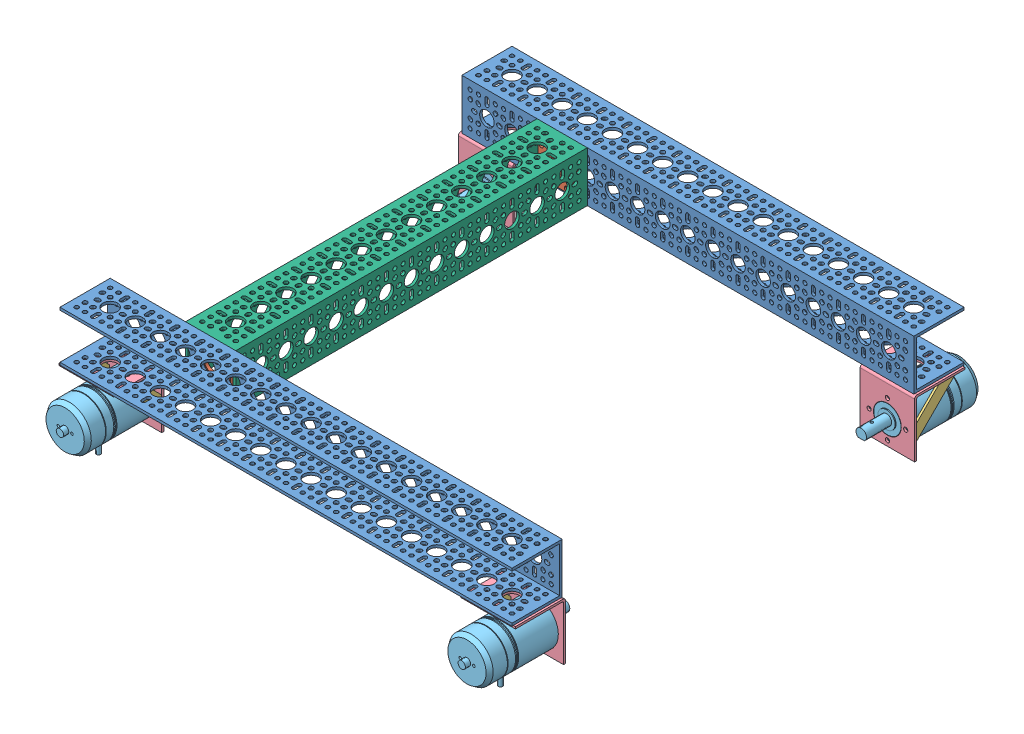
SolidWorks assembly 底座, configuration 默认. Lengths in mm.
Overall size (436 106 480.1).
19 component instances, 6 part files, 42 mates.
Components (placement in the parent):
- 432mm-U型梁-1: 432mm-U型梁 [默认] at (287.5256 66.9885 550.3792) x (0 -1 0) z (0 0 -1) size (48 432 48)
- 电机转向座-1: 电机转向座 [默认] at (-48.4744 66.9885 547.8792) x (1 0 0) z (0 1 0) size (43.24 12.23 43.24)
- 电机连接支架-1: 电机连接支架 [默认] at (-121.081 29.9055 566.0121) x (0 0 -1) z (1 0 0) size (98.3 58 52)
  - 小兔电机连接支架02-1: 小兔电机连接支架02 [默认] at (-18.8303 11.0829 24.6066) size (36.21 36.21 2)
  - 小兔电机连接支架02-2: 小兔电机连接支架02 [默认] at (-18.8303 11.0829 -25.3934) size (36.21 36.21 2)
  - 小兔电机连接支架-1: 小兔电机连接支架 [默认] at (17.3829 -18.9171 0.6066) size (48 54.5 52)
  - 3508无刷电机带减速箱（00）-1: 3508无刷电机带减速箱（00） [默认] at (-10.2171 -18.9171 0.6066) x (0 0 1) z (0 -1 0) size (42 98.3 47)
- 432mm-U型梁-2: 432mm-U型梁 [默认] at (-144.4744 66.9885 209.3792) x (0 -1 0) z (0 0 1) size (48 432 48)
- 电机转向座-2: 电机转向座 [默认] at (-48.4744 66.9885 211.8792) x (0 -1 0) z (-1 0 0) size (43.24 12.23 43.24)
- 小兔电机连接支架-1: 小兔电机连接支架 [默认] at (-120.4744 10.9885 211.1292) x (0 0 1) z (-1 0 0) size (48 54.5 52)
- 3508无刷电机带减速箱（00）-1: 3508无刷电机带减速箱（00） [默认] at (-120.4744 10.9885 183.5292) x (-1 0 0) z (0 -1 0) size (42 98.3 47)
- 小兔电机连接支架02-1: 小兔电机连接支架02 [默认] at (-94.4744 40.9885 174.916) x (0 0 1) z (-1 0 0) size (36.21 36.21 2)
- 小兔电机连接支架-2: 小兔电机连接支架 [默认] at (263.5256 10.9885 548.6292) x (0 0 -1) z (1 0 0) size (48 54.5 52)
- 3508无刷电机带减速箱（00）-2: 3508无刷电机带减速箱（00） [默认] at (263.5256 10.9885 576.2292) x (1 0 0) z (0 -1 0) size (42 98.3 47)
- 小兔电机连接支架02-2: 小兔电机连接支架02 [默认] at (237.5256 40.9885 584.8424) x (0 0 -1) z (1 0 0) size (36.21 36.21 2)
- 小兔电机连接支架-3: 小兔电机连接支架 [默认] at (263.5256 10.9885 211.1292) x (0 0 1) z (-1 0 0) size (48 54.5 52)
- 3508无刷电机带减速箱（00）-3: 3508无刷电机带减速箱（00） [默认] at (263.5256 10.9885 183.5292) x (-1 0 0) z (0 -1 0) size (42 98.3 47)
- 小兔电机连接支架02-3: 小兔电机连接支架02 [默认] at (289.5256 40.9885 174.916) x (0 0 1) z (-1 0 0) size (36.21 36.21 2)
- 336mm-U型梁-1: 336mm-U型梁 [默认] at (-48.4744 88.4885 547.8792) x (1 0 0) z (0 1 0) size (48 336 48)
Mates (geometry in assembly coordinates):
- Coincident4: coincident anti-aligned: plane of 432mm-U型梁-1 through (-144.4744 42.9885 547.8792) normal (0 0 -1); plane of 电机转向座-1 through (-48.4744 66.9885 547.8792) normal (0 0 1)
- Concentric3: concentric aligned: cylinder of 432mm-U型梁-1 through (-48.4744 66.9885 557.8792) axis (0 0 -1) radius 7; cylinder of 电机转向座-1 through (-48.4744 66.9885 547.8792) axis (0 0 -1) radius 7
- Concentric4: concentric aligned: cylinder of 432mm-U型梁-1 through (-40.4744 50.9885 557.8792) axis (0 0 -1) radius 2; cylinder of 电机转向座-1 through (-40.4744 50.9885 543.8792) axis (0 0 -1) radius 2
- Concentric5: concentric anti-aligned: cylinder of 432mm-U型梁-1 through (-120.4744 52.9885 571.8792) axis (0 -1 0) radius 7; cylinder of 电机连接支架-1/小兔电机连接支架-1 through (-120.4744 -11.5115 571.8792) axis (0 1 0) radius 7
- Coincident6: coincident anti-aligned: plane of 432mm-U型梁-1 through (-144.4744 42.9885 595.8792) normal (0 -1 0); plane of 电机连接支架-1/小兔电机连接支架-1 through (-146.4744 42.9885 594.6292) normal (0 1 0)
- Concentric6: concentric anti-aligned: cylinder of 432mm-U型梁-1 through (-136.4744 52.9885 587.8792) axis (0 -1 0) radius 2; cylinder of 电机连接支架-1/小兔电机连接支架-1 through (-136.4744 -11.5115 587.8792) axis (0 1 0) radius 2
- Coincident8: coincident anti-aligned: plane of 432mm-U型梁-2 through (287.5256 42.9885 211.8792) normal (0 0 1); plane of 电机转向座-2 through (-48.4744 66.9885 211.8792) normal (0 0 -1)
- Concentric9: concentric aligned: cylinder of 432mm-U型梁-2 through (-48.4744 66.9885 201.8792) axis (0 0 1) radius 7; cylinder of 电机转向座-2 through (-48.4744 66.9885 211.8792) axis (0 0 1) radius 7
- Coincident10: coincident aligned: plane of 小兔电机连接支架-1 through (-94.4744 40.9885 213.1292) normal (1 0 0); plane of 小兔电机连接支架02-1 through (-94.4744 40.9885 174.916) normal (1 0 0)
- Coincident11: coincident anti-aligned: plane of 小兔电机连接支架-1 through (-146.4744 40.9885 165.1292) normal (0 -1 0); plane of 小兔电机连接支架02-1 through (-96.4744 40.9885 174.916) normal (0 1 0)
- Coincident12: coincident anti-aligned: plane of 小兔电机连接支架-1 through (-120.4744 10.9885 211.1292) normal (0 0 -1); plane of 小兔电机连接支架02-1 through (-96.4744 19.7753 211.1292) normal (0 0 1)
- Coincident13: coincident anti-aligned: plane of 小兔电机连接支架-1 through (-120.4744 10.9885 211.1292) normal (0 0 -1); plane of 3508无刷电机带减速箱（00）-1 through (-133.4744 10.9885 211.1292) normal (0 0 1)
- Concentric10: concentric aligned: cylinder of 小兔电机连接支架-1 through (-120.4744 10.9885 213.1292) axis (0 0 -1) radius 13.25; cylinder of 3508无刷电机带减速箱（00）-1 through (-120.4744 10.9885 174.8292) axis (0 0 -1) radius 13
- Concentric11: concentric anti-aligned: cylinder of 小兔电机连接支架-1 through (-102.9744 10.9885 213.1292) axis (0 0 -1) radius 2; cylinder of 3508无刷电机带减速箱（00）-1 through (-102.9744 10.9885 211.1292) axis (0 0 1) radius 1.65
- Concentric12: concentric anti-aligned: cylinder of 432mm-U型梁-2 through (-120.4744 52.9885 187.8792) axis (0 -1 0) radius 7; cylinder of 小兔电机连接支架-1 through (-120.4744 -11.5115 187.8792) axis (0 1 0) radius 7
- Coincident14: coincident anti-aligned: plane of 432mm-U型梁-2 through (287.5256 42.9885 163.8792) normal (0 -1 0); plane of 小兔电机连接支架-1 through (-94.4744 42.9885 165.1292) normal (0 1 0)
- Concentric14: concentric anti-aligned: cylinder of 432mm-U型梁-2 through (-136.4744 52.9885 171.8792) axis (0 -1 0) radius 2; cylinder of 小兔电机连接支架-1 through (-136.4744 -11.5115 171.8792) axis (0 1 0) radius 2
- Coincident15: coincident aligned: plane of 小兔电机连接支架-2 through (237.5256 40.9885 546.6292) normal (-1 0 0); plane of 小兔电机连接支架02-2 through (237.5256 40.9885 584.8424) normal (-1 0 0)
- Coincident16: coincident anti-aligned: plane of 小兔电机连接支架-2 through (289.5256 40.9885 594.6292) normal (0 -1 0); plane of 小兔电机连接支架02-2 through (239.5256 40.9885 584.8424) normal (0 1 0)
- Coincident17: coincident anti-aligned: plane of 小兔电机连接支架-2 through (263.5256 10.9885 548.6292) normal (0 0 1); plane of 小兔电机连接支架02-2 through (239.5256 19.7753 548.6292) normal (0 0 -1)
- Coincident18: coincident anti-aligned: plane of 小兔电机连接支架-2 through (263.5256 10.9885 548.6292) normal (0 0 1); plane of 3508无刷电机带减速箱（00）-2 through (276.5256 10.9885 548.6292) normal (0 0 -1)
- Concentric15: concentric aligned: cylinder of 小兔电机连接支架-2 through (263.5256 10.9885 546.6292) axis (0 0 1) radius 13.25; cylinder of 3508无刷电机带减速箱（00）-2 through (263.5256 10.9885 584.9292) axis (0 0 1) radius 13
- Concentric16: concentric anti-aligned: cylinder of 小兔电机连接支架-2 through (246.0256 10.9885 546.6292) axis (0 0 1) radius 2; cylinder of 3508无刷电机带减速箱（00）-2 through (246.0256 10.9885 548.6292) axis (0 0 -1) radius 1.65
- Coincident19: coincident aligned: plane of 小兔电机连接支架-3 through (289.5256 40.9885 213.1292) normal (1 0 0); plane of 小兔电机连接支架02-3 through (289.5256 40.9885 174.916) normal (1 0 0)
- Coincident20: coincident anti-aligned: plane of 小兔电机连接支架-3 through (237.5256 40.9885 165.1292) normal (0 -1 0); plane of 小兔电机连接支架02-3 through (287.5256 40.9885 174.916) normal (0 1 0)
- Coincident21: coincident anti-aligned: plane of 小兔电机连接支架-3 through (263.5256 10.9885 211.1292) normal (0 0 -1); plane of 小兔电机连接支架02-3 through (287.5256 19.7753 211.1292) normal (0 0 1)
- Coincident22: coincident anti-aligned: plane of 小兔电机连接支架-3 through (263.5256 10.9885 211.1292) normal (0 0 -1); plane of 3508无刷电机带减速箱（00）-3 through (250.5256 10.9885 211.1292) normal (0 0 1)
- Concentric17: concentric aligned: cylinder of 小兔电机连接支架-3 through (263.5256 10.9885 213.1292) axis (0 0 -1) radius 13.25; cylinder of 3508无刷电机带减速箱（00）-3 through (263.5256 10.9885 174.8292) axis (0 0 -1) radius 13
- Concentric18: concentric anti-aligned: cylinder of 小兔电机连接支架-3 through (281.0256 10.9885 213.1292) axis (0 0 -1) radius 2; cylinder of 3508无刷电机带减速箱（00）-3 through (281.0256 10.9885 211.1292) axis (0 0 1) radius 1.65
- Concentric19: concentric anti-aligned: cylinder of 432mm-U型梁-1 through (263.5256 52.9885 571.8792) axis (0 -1 0) radius 7; cylinder of 小兔电机连接支架-2 through (263.5256 -11.5115 571.8792) axis (0 1 0) radius 7
- Coincident23: coincident anti-aligned: plane of 432mm-U型梁-1 through (-144.4744 42.9885 595.8792) normal (0 -1 0); plane of 小兔电机连接支架-2 through (237.5256 42.9885 594.6292) normal (0 1 0)
- Concentric20: concentric anti-aligned: cylinder of 432mm-U型梁-1 through (279.5256 52.9885 587.8792) axis (0 -1 0) radius 2; cylinder of 小兔电机连接支架-2 through (279.5256 -11.5115 587.8792) axis (0 1 0) radius 2
- Concentric21: concentric anti-aligned: cylinder of 432mm-U型梁-2 through (263.5256 52.9885 187.8792) axis (0 -1 0) radius 7; cylinder of 小兔电机连接支架-3 through (263.5256 -11.5115 187.8792) axis (0 1 0) radius 7
- Coincident24: coincident anti-aligned: plane of 432mm-U型梁-2 through (287.5256 42.9885 163.8792) normal (0 -1 0); plane of 小兔电机连接支架-3 through (289.5256 42.9885 165.1292) normal (0 1 0)
- Concentric22: concentric anti-aligned: cylinder of 432mm-U型梁-2 through (279.5256 52.9885 171.8792) axis (0 -1 0) radius 2; cylinder of 小兔电机连接支架-3 through (279.5256 -11.5115 171.8792) axis (0 1 0) radius 2
- Coincident25: coincident aligned: plane of 432mm-U型梁-1 through (-144.4744 90.9885 595.8792) normal (0 1 0); plane of 336mm-U型梁-1 through (-24.4744 90.9885 211.8792) normal (0 1 0)
- Coincident26: coincident anti-aligned: plane of 432mm-U型梁-1 through (-144.4744 42.9885 547.8792) normal (0 0 -1); plane of 336mm-U型梁-1 through (-48.4744 88.4885 547.8792) normal (0 0 1)
- Coincident27: coincident anti-aligned: plane of 电机转向座-1 through (-26.9744 66.9885 543.8792) normal (1 0 0); plane of 336mm-U型梁-1 through (-26.9744 88.4885 211.8792) normal (-1 0 0)
- Concentric23: concentric anti-aligned: cone of 电机转向座-1 through (-26.9744 82.9885 539.8792) axis (-1 0 0); cylinder of 336mm-U型梁-1 through (-34.4744 82.9885 539.8792) axis (1 0 0) radius 2
- Coincident28: coincident anti-aligned: plane of 电机转向座-2 through (-69.9744 66.9885 202.6868) normal (-1 0 0); plane of 336mm-U型梁-1 through (-69.9744 88.4885 211.8792) normal (1 0 0)
- Concentric24: concentric anti-aligned: cone of 电机转向座-2 through (-69.9744 82.9885 219.8792) axis (1 0 0); cylinder of 336mm-U型梁-1 through (-62.4744 82.9885 219.8792) axis (-1 0 0) radius 2
- Concentric25: concentric anti-aligned: cone of 电机转向座-2 through (-69.9744 50.9885 219.8792) axis (1 0 0); cylinder of 336mm-U型梁-1 through (-62.4744 50.9885 219.8792) axis (-1 0 0) radius 2
